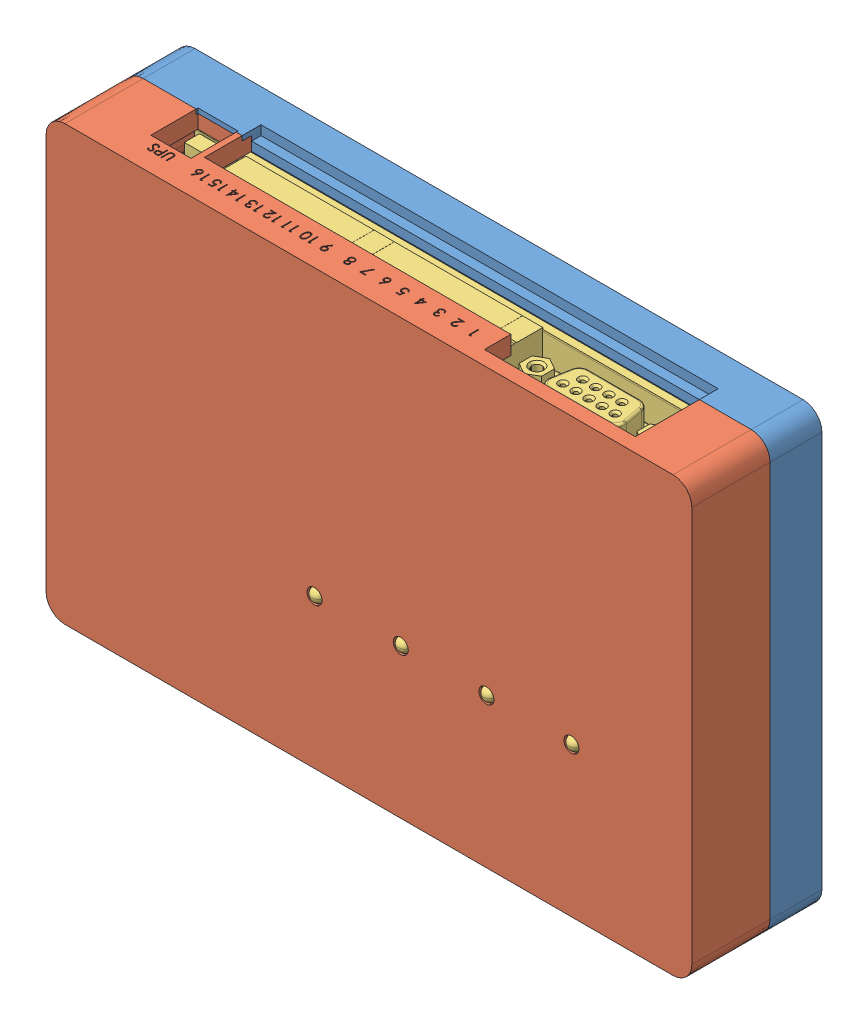
SolidWorks assembly CTL1, configuration Default. Lengths in mm.
Overall size (137 92 28.17).
3 component instances, 3 part files, 5 mates.
Components (placement in the parent):
- Controller_p1_edit3-1: Controller_p1_edit3 [Default] at (-123.6302 -57.7804 31.5949) size (137 92 11)
- Controller_p2_edit1-1: Controller_p2_edit1 [Default] at (-123.6302 34.2196 58.1949) x (1 0 0) z (0 0 -1) size (137 92 18.6)
- controller1-1: controller1 [Default] at (-114.5451 -53.6916 42.219) size (118.81 84.36 21.8)
Mates (geometry in assembly coordinates):
- Coincident6: coincident: plane of assembly; plane of assembly; plane of Controller_p1_edit3-1 through (-122.6302 -56.7804 42.5949) normal (0 1 0); plane of Controller_p2_edit1-1 through (-122.6302 -56.7804 42.5949) normal (0 -1 0)
- Coincident7: coincident: plane of assembly; plane of assembly; plane of Controller_p1_edit3-1 through (-122.6302 -56.7804 42.5949) normal (1 0 0); plane of Controller_p2_edit1-1 through (-122.6302 33.2196 42.5949) normal (-1 0 0)
- Coincident8: coincident: plane of assembly; plane of assembly; plane of Controller_p1_edit3-1 through (-123.6302 -57.7804 40.5949) normal (0 0 1); plane of controller1-1 through (-114.5451 -53.6916 40.5949) normal (0 0 -1)
- Concentric1: concentric: cylinder of assembly; cylinder of assembly; cylinder of Controller_p1_edit3-1 through (-112.6302 28.2196 40.5949) axis (0 0 -1) radius 1.35; cylinder of controller1-1 through (-112.6302 28.2196 40.2193) axis (0 0 1) radius 1.5
- Coincident9: coincident: plane of assembly; plane of assembly; plane of Controller_p1_edit3-1 through (-123.6302 -57.7804 40.5949) normal (0 0 1); plane of Controller_p2_edit1-1 through (-123.6302 34.2196 40.5949) normal (0 0 -1)
